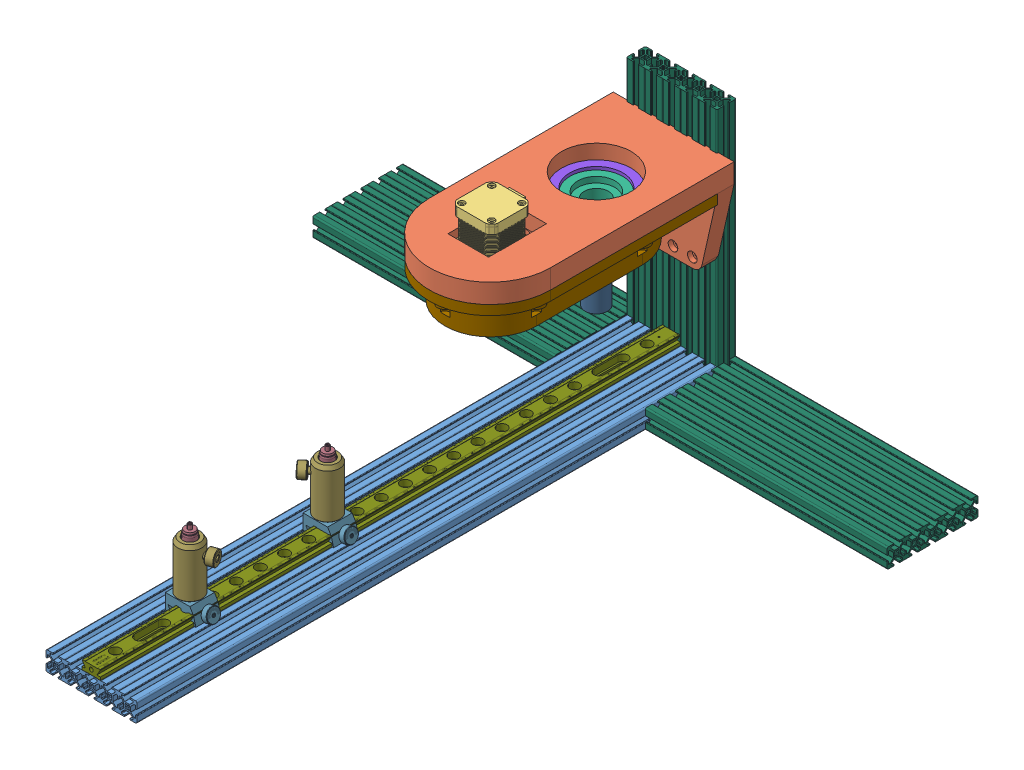
SolidWorks assembly OpenCALAssembly.v3, configuration Default. Lengths in mm.
Overall size (594 250 620.03).
27 component instances, 18 part files, 27 mates.
Components (placement in the parent):
- 20-2020-Black-25-CL.stp-1: 20-2020-Black-25-CL.stp [Default] at (5.4558 13.0651 39.4201) size (94 20 600)
- VerticalStageAssembly.v2-1: VerticalStageAssembly.v2 [Default] at (29.9175 152.6715 -478.4666) x (0 0 -1) z (1 0 0) size (252.5 145.51 125)
  - VerticalStage-1: VerticalStage [Default] at (83.6132 -98.677 -49.2178) size (252.5 100 125)
  - Assem3^VerticalStageAssembly.v2-1: Assem3^VerticalStageAssembly.v2 [Default] at origin size (166.51 64.5 74) (virtual)
    - Copy of Assem2^Assem3_VerticalStageAssembly.v2-1: Copy of Assem2^Assem3_VerticalStageAssembly.v2 [Default] at origin size (47.8 64.5 42.3) (virtual)
      - Nema17-1: Nema17 [Predeterminado] at (-104.7481 84.323 13.4322) x (0 0 1) z (1 0 0) size (42.3 64.5 47.8)
      - T5 Pulley-1: T5 Pulley [Predeterminado] at (-104.7481 37.623 13.4322) x (0 -1 0) z (0 0 1) size (14.8 16 16)
    - Belt-1: Belt [Default] at (-108.6865 25.623 13.493) size (153.36 6 74)
  - Assem1^VerticalStageAssembly.v2-1: Assem1^VerticalStageAssembly.v2 [Default] at origin size (98.27 60.66 98.27) (virtual)
    - er32 x 34ths ToolHolderOpenCAL-1: er32 x 34ths ToolHolderOpenCAL [Default] at (-15.7823 32.6902 -13.7293) x (0.420729 0 0.907186) z (0.907186 0 -0.420729) size (74 44.7 74)
    - ER32 COLLET NUT-1: ER32 COLLET NUT [Default] at (3.8533 13.4515 11.5736) x (0 -1 0) z (0.99027 0 0.13916) size (22.61 50 50) (hidden)
    - ER32-20.step-1: ER32-20.step [Default] at (3.6132 -14.2638 13.2822) x (0.698361 0 0.715746) z (0 -1 0) size (32.96 32.96 40.01)
    - BallBearing-1: BallBearing [Default] at (3.6132 11.6902 13.2822) x (0.999353 0 0.035955) z (-0.035955 0 0.999353) size (72 9 72)
    - BallBearing-2: BallBearing [Default] at (3.6132 46.3902 13.2822) x (-0.871455 0 -0.490475) z (-0.490475 0 0.871455) size (72 9 72)
  - ColletStageHousing-1: ColletStageHousing [Default] at (3.6132 1.3202 13.2822) x (0 1 0) z (0 0 -1) size (40 235.5 125)
  - Vial (20mm)-1: Vial (20mm) [Default] at (3.6132 -56.6823 13.2822) x (0.222456 0 0.974943) z (-0.974943 0 0.222456) size (23 41.5 23)
  - Spacer-1: Spacer [Default] at (3.6132 8.8202 13.2822) size (75 2.87 75)
- PH50_M-Solidworks-1: PH50_M-Solidworks [Default] at (39.4918 57.7304 -72.239) x (-0.331511 0 -0.943451) z (0.943451 0 -0.331511) size (25 50.44 35.14)
- TR75_M-Solidworks-1: TR75_M-Solidworks [Default] at (34.6119 20.7616 -70.2602) x (0.667274 0 0.744812) z (-0.744812 0 0.667274) size (12.67 80.02 12.87)
- RC1-Solidworks-1: RC1-Solidworks [Default] at (53.5095 23.0651 -57.5602) x (0 0 -1) z (1 0 0) size (25.4 16.53 39.23)
- 20-2020-Black-25-CLShort.stp-1: 20-2020-Black-25-CLShort.stp [Default] at (-4.5442 13.0651 -496.5799) x (0 0 -1) z (1 0 0) size (94 20 250)
- 20-2020-Black-25-CLShort.stp-2: 20-2020-Black-25-CLShort.stp [Default] at (339.4558 13.0651 -496.5799) x (0 0 -1) z (1 0 0) size (94 20 250)
- PH50_M-Solidworks-2: PH50_M-Solidworks [Default] at (30.7203 57.7304 -209.1749) x (0.637938 0 0.770088) z (-0.770088 0 0.637938) size (25 50.44 35.14)
- TR75_M-Solidworks-2: TR75_M-Solidworks [Default] at (34.6119 19.9745 -212.7222) x (0.321219 0 0.947005) z (-0.947005 0 0.321219) size (12.67 80.02 12.87)
- RC1-Solidworks-2: RC1-Solidworks [Default] at (53.5095 23.0651 -200.0222) x (0 0 -1) z (1 0 0) size (25.4 16.53 39.23)
- RLA600_M-Solidworks-1: RLA600_M-Solidworks [Default] at (42.2404 28.1451 -260.5528) size (19.05 9.53 600)
- 20-2020-Black-25-CLShort.stp-4: 20-2020-Black-25-CLShort.stp [Default] at (79.4558 253.0651 -570.5799) x (-1 0 0) z (0 1 0) size (94 20 250)
Mates (geometry in assembly coordinates):
- Concentric1: concentric aligned: circle of PH50_M-Solidworks-1; cylinder of TR75_M-Solidworks-1 through (34.6119 95.7678 -70.2602) axis (0 1 0) radius 6.3373
- Concentric2: concentric anti-aligned: circle of PH50_M-Solidworks-1; circle of RC1-Solidworks-1
- Coincident4: coincident anti-aligned: plane of PH50_M-Solidworks-1 through (43.7754 38.5591 -44.1819) normal (0 -1 0); plane of RC1-Solidworks-1 through (21.9119 38.5591 -57.5602) normal (0 1 0)
- Parallel1: parallel aligned: plane of 20-2020-Black-25-CL.stp-1 through (-3.0442 4.5651 39.4201) normal (0 0 1); plane of RC1-Solidworks-1 through (21.9119 23.0651 -57.5602) normal (0 0 1)
- Coincident6: coincident aligned: line of 20-2020-Black-25-CL.stp-1 through (45.5938 23.0651 -560.5799) axis (0 0 1); line of RC1-Solidworks-1 through (45.5938 23.0651 -82.9602) axis (0 0 1)
- Coincident7: coincident anti-aligned: plane of 20-2020-Black-25-CL.stp-1 through (32.4558 23.0651 14.4201) normal (0 1 0); plane of RC1-Solidworks-1 through (21.9119 23.0651 -57.5602) normal (0 -1 0)
- Coincident13: coincident anti-aligned: plane of 20-2020-Black-25-CL.stp-1 through (89.4558 4.5651 14.4201) normal (1 0 0); plane of 20-2020-Black-25-CL.stp-3 through (89.4558 13.0651 -350.9237) normal (-1 0 0)
- Coincident15: coincident anti-aligned: plane of 20-2020-Black-25-CL.stp-1 through (-4.5442 21.5651 14.4201) normal (-1 0 0); plane of 20-2020-Black-25-CL.stp-4 through (-4.5442 4.5651 -488.0799) normal (1 0 0)
- Coincident19: coincident aligned: plane of 20-2020-Black-25-CLShort.stp-1 through (-29.5442 4.5651 -580.5799) normal (0 0 -1); plane of 20-2020-Black-25-CLShort.stp-2 through (314.4558 16.2031 -580.5799) normal (0 0 -1)
- Coincident20: coincident anti-aligned: plane of 20-2020-Black-25-CL.stp-1 through (89.4558 16.2031 14.4201) normal (1 0 0); plane of 20-2020-Black-25-CLShort.stp-2 through (89.4558 13.0651 -496.5799) normal (-1 0 0)
- Concentric3: concentric aligned: circle of PH50_M-Solidworks-2; cylinder of TR75_M-Solidworks-2 through (34.6119 94.9807 -212.7222) axis (0 1 0) radius 6.3373
- Concentric4: concentric anti-aligned: circle of PH50_M-Solidworks-2; circle of RC1-Solidworks-2
- Coincident21: coincident anti-aligned: plane of PH50_M-Solidworks-2 through (16.9784 38.5591 -234.0085) normal (0 -1 0); plane of RC1-Solidworks-2 through (21.9119 38.5591 -200.0222) normal (0 1 0)
- Parallel2: parallel aligned: plane of 20-2020-Black-25-CL.stp-1 through (-3.0442 4.5651 39.4201) normal (0 0 1); plane of RC1-Solidworks-2 through (21.9119 23.0651 -200.0222) normal (0 0 1)
- Coincident22: coincident aligned: line of 20-2020-Black-25-CL.stp-1 through (45.5938 23.0651 -560.5799) axis (0 0 1); line of RC1-Solidworks-2 through (45.5938 23.0651 -225.4222) axis (0 0 1)
- Coincident23: coincident anti-aligned: plane of 20-2020-Black-25-CL.stp-1 through (32.4558 23.0651 14.4201) normal (0 1 0); plane of RC1-Solidworks-2 through (21.9119 23.0651 -200.0222) normal (0 -1 0)
- Parallel4: parallel anti-aligned: line of 20-2020-Black-25-CL.stp-1 through (50.9558 23.0651 39.4201) axis (-1 0 0); line of RLA600_M-Solidworks-1 through (35.9158 23.3191 39.4472) axis (1 0 0)
- Coincident28: coincident anti-aligned: plane of 20-2020-Black-25-CL.stp-1 through (50.9558 23.0651 14.4201) normal (0 1 0); plane of RLA600_M-Solidworks-1 through (51.7654 23.0651 39.4472) normal (0 -1 0)
- Coincident36: coincident anti-aligned: plane of 20-2020-Black-25-CL.stp-1 through (5.4558 13.0651 -560.5799) normal (0 0 -1); plane of 20-2020-Black-25-CLShort.stp-4 through (-3.0442 228.0651 -560.5799) normal (0 0 1)
- Coincident37: coincident aligned: line of 20-2020-Black-25-CL.stp-1 through (-3.0442 3.0651 -560.5799) axis (1 0 0); line of 20-2020-Black-25-CLShort.stp-4 through (8.5938 3.0651 -560.5799) axis (1 0 0)
- Coincident38: coincident aligned: plane of 20-2020-Black-25-CL.stp-1 through (-4.5442 9.9271 14.4201) normal (-1 0 0); plane of 20-2020-Black-25-CLShort.stp-4 through (-4.5442 228.0651 -567.4419) normal (-1 0 0)
- Coincident45: coincident: point of VerticalStageAssembly.v2-1/VerticalStage-1; line of 20-2020-Black-25-CLShort.stp-4 through (89.4558 3.0651 -562.0799) axis (0 1 0)
- Parallel8: parallel aligned: plane of VerticalStageAssembly.v2-1/VerticalStage-1 through (105.6997 213.9945 -562.0799) normal (0 1 0); plane of 20-2020-Black-25-CLShort.stp-4 through (87.9558 253.0651 -579.0799) normal (0 1 0)
- Parallel9: parallel anti-aligned: plane of VerticalStageAssembly.v2-1/VerticalStage-1 through (105.6997 53.9945 -562.0799) normal (0 0 -1); plane of 20-2020-Black-25-CLShort.stp-4 through (-3.0442 228.0651 -560.5799) normal (0 0 1)
- Coincident48: coincident aligned: plane of 20-2020-Black-25-CLShort.stp-2 through (314.4558 16.2031 -580.5799) normal (0 0 -1); plane of 20-2020-Black-25-CLShort.stp-4 through (87.9558 228.0651 -580.5799) normal (0 0 -1)
- Coincident49: coincident aligned: plane of 20-2020-Black-25-CLShort.stp-2 through (314.4558 3.0651 -573.7179) normal (0 -1 0); plane of 20-2020-Black-25-CLShort.stp-4 through (79.4558 3.0651 -570.5799) normal (0 -1 0)
- Coincident50: coincident aligned: plane of 20-2020-Black-25-CLShort.stp-1 through (-29.5442 3.0651 -573.7179) normal (0 -1 0); plane of 20-2020-Black-25-CLShort.stp-4 through (79.4558 3.0651 -570.5799) normal (0 -1 0)
